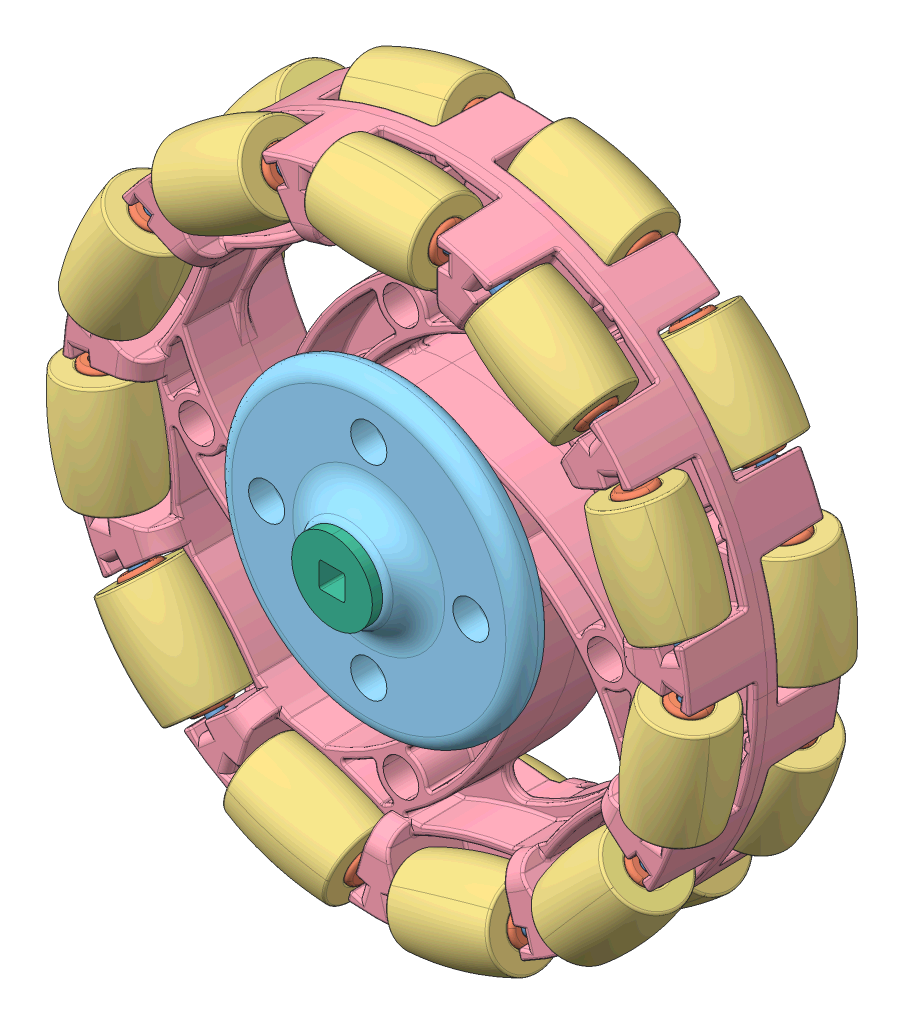
SolidWorks assembly Holo_Module_Omni_Wheel_Assembly, configuration Default. Lengths in mm.
Overall size (90.82 89.11 34).
95 component instances, 6 part files, 12 mates.
Components (placement in the parent):
- 3.25_ Omni-Directional Wheel (276-3526) part-1: 3.25_ Omni-Directional Wheel (276-3526) part [Default] at (20.7471 51.0724 74.1563) size (90.82 89.11 34)
  - 3.25_ Omni-Directional Wheel (276-3526) .step-1: 3.25_ Omni-Directional Wheel (276-3526) .step [Default] at origin size (90.82 89.11 34)
    - Roller Assembly.step-1: Roller Assembly.step [Default] at (-0.0014 35.9575 7.1) x (0 0.963098 -0.269151) z (-1 0 0) size (14.05 14.05 18.75)
      - 276-3526-001 Rev 1.step-1: 276-3526-001 Rev 1.step [Default] at origin size (2 2 18.75)
      - 276-3526-003 Rev 1.step-1: 276-3526-003 Rev 1.step [Default] at origin size (6.15 6.15 14.2)
      - 276-3526-002 Rev 1.step-1: 276-3526-002 Rev 1.step [Default] x (0 0 1) z (-0.908956 0.416893 0) size (13.2 10.6 10.6)
    - Roller Assembly.step-2: Roller Assembly.step [Default] at (-19.4287 30.2567 7.1) x (0.421057 -0.655178 0.627258) z (-0.841254 -0.540641 0) size (14.05 14.05 18.75)
      - 276-3526-001 Rev 1.step-1: 276-3526-001 Rev 1.step [Default] at origin size (2 2 18.75)
      - 276-3526-003 Rev 1.step-1: 276-3526-003 Rev 1.step [Default] at origin size (6.15 6.15 14.2)
      - 276-3526-002 Rev 1.step-1: 276-3526-002 Rev 1.step [Default] x (0 0 1) z (-0.908956 0.416893 0) size (13.2 10.6 10.6)
    - Roller Assembly.step-3: Roller Assembly.step [Default] at (-35.5935 -5.1038 7.1) x (0.979746 0.140866 -0.142315) z (0.142315 -0.989821 0) size (14.05 14.05 18.75)
      - 276-3526-001 Rev 1.step-1: 276-3526-001 Rev 1.step [Default] at origin size (2 2 18.75)
      - 276-3526-003 Rev 1.step-1: 276-3526-003 Rev 1.step [Default] at origin size (6.15 6.15 14.2)
      - 276-3526-002 Rev 1.step-1: 276-3526-002 Rev 1.step [Default] x (0 0 1) z (-0.908956 0.416893 0) size (13.2 10.6 10.6)
    - Roller Assembly.step-4: Roller Assembly.step [Default] at (-10.1434 -34.4972 7.1) x (0.079373 0.27032 -0.959493) z (0.959493 -0.281733 0) size (14.05 14.05 18.75)
      - 276-3526-001 Rev 1.step-1: 276-3526-001 Rev 1.step [Default] at origin size (2 2 18.75)
      - 276-3526-003 Rev 1.step-1: 276-3526-003 Rev 1.step [Default] at origin size (6.15 6.15 14.2)
      - 276-3526-002 Rev 1.step-1: 276-3526-002 Rev 1.step [Default] x (0 0 1) z (-0.908956 0.416893 0) size (13.2 10.6 10.6)
    - Roller Assembly.step-5: Roller Assembly.step [Default] at (27.166 -23.5574 7.1) x (-0.355209 0.30779 -0.882662) z (0.654861 0.75575 0) size (14.05 14.05 18.75)
      - 276-3526-001 Rev 1.step-1: 276-3526-001 Rev 1.step [Default] at origin size (2 2 18.75)
      - 276-3526-003 Rev 1.step-1: 276-3526-003 Rev 1.step [Default] at origin size (6.15 6.15 14.2)
      - 276-3526-002 Rev 1.step-1: 276-3526-002 Rev 1.step [Default] x (0 0 1) z (-0.908956 0.416893 0) size (13.2 10.6 10.6)
    - Roller Assembly.step-6: Roller Assembly.step [Default] at (32.7138 14.9249 7.1) x (0.89908 0.410596 0.151875) z (-0.415415 0.909632 0) size (14.05 14.05 18.75)
      - 276-3526-001 Rev 1.step-1: 276-3526-001 Rev 1.step [Default] at origin size (2 2 18.75)
      - 276-3526-003 Rev 1.step-1: 276-3526-003 Rev 1.step [Default] at origin size (6.15 6.15 14.2)
      - 276-3526-002 Rev 1.step-1: 276-3526-002 Rev 1.step [Default] x (0 0 1) z (-0.908956 0.416893 0) size (13.2 10.6 10.6)
    - Roller Assembly.step-7: Roller Assembly.step [Default] at (19.4515 30.242 7.1) x (0.194707 0.302971 0.932898) z (-0.841254 0.540641 0) size (14.05 14.05 18.75)
      - 276-3526-001 Rev 1.step-1: 276-3526-001 Rev 1.step [Default] at origin size (2 2 18.75)
      - 276-3526-003 Rev 1.step-1: 276-3526-003 Rev 1.step [Default] at origin size (6.15 6.15 14.2)
      - 276-3526-002 Rev 1.step-1: 276-3526-002 Rev 1.step [Default] x (0 0 1) z (-0.908956 0.416893 0) size (13.2 10.6 10.6)
    - Roller Assembly.step-8: Roller Assembly.step [Default] at (-32.7025 14.9497 7.1) x (0.82743 -0.377875 0.415415) z (-0.415415 -0.909632 0) size (14.05 14.05 18.75)
      - 276-3526-001 Rev 1.step-1: 276-3526-001 Rev 1.step [Default] at origin size (2 2 18.75)
      - 276-3526-003 Rev 1.step-1: 276-3526-003 Rev 1.step [Default] at origin size (6.15 6.15 14.2)
      - 276-3526-002 Rev 1.step-1: 276-3526-002 Rev 1.step [Default] x (0 0 1) z (-0.908956 0.416893 0) size (13.2 10.6 10.6)
    - Roller Assembly.step-9: Roller Assembly.step [Default] at (-27.1838 -23.5369 7.1) x (0.578931 0.501646 -0.642799) z (0.654861 -0.75575 0) size (14.05 14.05 18.75)
      - 276-3526-001 Rev 1.step-1: 276-3526-001 Rev 1.step [Default] at origin size (2 2 18.75)
      - 276-3526-003 Rev 1.step-1: 276-3526-003 Rev 1.step [Default] at origin size (6.15 6.15 14.2)
      - 276-3526-002 Rev 1.step-1: 276-3526-002 Rev 1.step [Default] x (0 0 1) z (-0.908956 0.416893 0) size (13.2 10.6 10.6)
    - Roller Assembly.step-10: Roller Assembly.step [Default] at (10.1174 -34.5048 7.1) x (0.079373 -0.27032 -0.959493) z (0.959493 0.281733 0) size (14.05 14.05 18.75)
      - 276-3526-001 Rev 1.step-1: 276-3526-001 Rev 1.step [Default] at origin size (2 2 18.75)
      - 276-3526-003 Rev 1.step-1: 276-3526-003 Rev 1.step [Default] at origin size (6.15 6.15 14.2)
      - 276-3526-002 Rev 1.step-1: 276-3526-002 Rev 1.step [Default] x (0 0 1) z (-0.908956 0.416893 0) size (13.2 10.6 10.6)
    - Roller Assembly.step-11: Roller Assembly.step [Default] at (35.5896 -5.1307 7.1) x (0.988515 -0.142127 -0.05136) z (0.142315 0.989821 0) size (14.05 14.05 18.75)
      - 276-3526-001 Rev 1.step-1: 276-3526-001 Rev 1.step [Default] at origin size (2 2 18.75)
      - 276-3526-003 Rev 1.step-1: 276-3526-003 Rev 1.step [Default] at origin size (6.15 6.15 14.2)
      - 276-3526-002 Rev 1.step-1: 276-3526-002 Rev 1.step [Default] x (0 0 1) z (-0.908956 0.416893 0) size (13.2 10.6 10.6)
    - Roller Assembly.step-12: Roller Assembly.step [Default] at (10.1434 34.4972 -7.1) x (0.083119 0.283078 -0.955489) z (0.959493 -0.281733 0) size (14.05 14.05 18.75)
      - 276-3526-001 Rev 1.step-1: 276-3526-001 Rev 1.step [Default] at origin size (2 2 18.75)
      - 276-3526-003 Rev 1.step-1: 276-3526-003 Rev 1.step [Default] at origin size (6.15 6.15 14.2)
      - 276-3526-002 Rev 1.step-1: 276-3526-002 Rev 1.step [Default] x (0 0 1) z (-0.908956 0.416893 0) size (13.2 10.6 10.6)
    - Roller Assembly.step-13: Roller Assembly.step [Default] at (27.1838 23.5369 -7.1) x (0.582526 0.504762 -0.637086) z (0.654861 -0.75575 0) size (14.05 14.05 18.75)
      - 276-3526-001 Rev 1.step-1: 276-3526-001 Rev 1.step [Default] at origin size (2 2 18.75)
      - 276-3526-003 Rev 1.step-1: 276-3526-003 Rev 1.step [Default] at origin size (6.15 6.15 14.2)
      - 276-3526-002 Rev 1.step-1: 276-3526-002 Rev 1.step [Default] x (0 0 1) z (-0.908956 0.416893 0) size (13.2 10.6 10.6)
    - Roller Assembly.step-14: Roller Assembly.step [Default] at (35.5935 5.1038 -7.1) x (0.926341 0.133188 -0.352355) z (0.142315 -0.989821 0) size (14.05 14.05 18.75)
      - 276-3526-001 Rev 1.step-1: 276-3526-001 Rev 1.step [Default] at origin size (2 2 18.75)
      - 276-3526-003 Rev 1.step-1: 276-3526-003 Rev 1.step [Default] at origin size (6.15 6.15 14.2)
      - 276-3526-002 Rev 1.step-1: 276-3526-002 Rev 1.step [Default] x (0 0 1) z (-0.908956 0.416893 0) size (13.2 10.6 10.6)
    - Roller Assembly.step-15: Roller Assembly.step [Default] at (32.7025 -14.9497 -7.1) x (0.897398 -0.409828 0.163453) z (-0.415415 -0.909632 0) size (14.05 14.05 18.75)
      - 276-3526-001 Rev 1.step-1: 276-3526-001 Rev 1.step [Default] at origin size (2 2 18.75)
      - 276-3526-003 Rev 1.step-1: 276-3526-003 Rev 1.step [Default] at origin size (6.15 6.15 14.2)
      - 276-3526-002 Rev 1.step-1: 276-3526-002 Rev 1.step [Default] x (0 0 1) z (-0.908956 0.416893 0) size (13.2 10.6 10.6)
    - Roller Assembly.step-16: Roller Assembly.step [Default] at (19.4287 -30.2567 -7.1) x (0.277612 -0.431972 0.858098) z (-0.841254 -0.540641 0) size (14.05 14.05 18.75)
      - 276-3526-001 Rev 1.step-1: 276-3526-001 Rev 1.step [Default] at origin size (2 2 18.75)
      - 276-3526-003 Rev 1.step-1: 276-3526-003 Rev 1.step [Default] at origin size (6.15 6.15 14.2)
      - 276-3526-002 Rev 1.step-1: 276-3526-002 Rev 1.step [Default] x (0 0 1) z (-0.908956 0.416893 0) size (13.2 10.6 10.6)
    - Roller Assembly.step-17: Roller Assembly.step [Default] at (-0.0136 -35.9575 -7.1) x (0 -0.239919 0.970793) z (-1 0 0) size (14.05 14.05 18.75)
      - 276-3526-001 Rev 1.step-1: 276-3526-001 Rev 1.step [Default] at origin size (2 2 18.75)
      - 276-3526-003 Rev 1.step-1: 276-3526-003 Rev 1.step [Default] at origin size (6.15 6.15 14.2)
      - 276-3526-002 Rev 1.step-1: 276-3526-002 Rev 1.step [Default] x (0 0 1) z (-0.908956 0.416893 0) size (13.2 10.6 10.6)
    - Roller Assembly.step-18: Roller Assembly.step [Default] at (-19.4515 -30.242 -7.1) x (0.31008 0.482494 0.819176) z (-0.841254 0.540641 0) size (14.05 14.05 18.75)
      - 276-3526-001 Rev 1.step-1: 276-3526-001 Rev 1.step [Default] at origin size (2 2 18.75)
      - 276-3526-003 Rev 1.step-1: 276-3526-003 Rev 1.step [Default] at origin size (6.15 6.15 14.2)
      - 276-3526-002 Rev 1.step-1: 276-3526-002 Rev 1.step [Default] x (0 0 1) z (-0.908956 0.416893 0) size (13.2 10.6 10.6)
    - Roller Assembly.step-19: Roller Assembly.step [Default] at (-32.7138 -14.9249 -7.1) x (0.58758 0.268339 0.763377) z (-0.415415 0.909632 0) size (14.05 14.05 18.75)
      - 276-3526-001 Rev 1.step-1: 276-3526-001 Rev 1.step [Default] at origin size (2 2 18.75)
      - 276-3526-003 Rev 1.step-1: 276-3526-003 Rev 1.step [Default] at origin size (6.15 6.15 14.2)
      - 276-3526-002 Rev 1.step-1: 276-3526-002 Rev 1.step [Default] x (0 0 1) z (-0.908956 0.416893 0) size (13.2 10.6 10.6)
    - Roller Assembly.step-20: Roller Assembly.step [Default] at (-35.5896 5.1307 -7.1) x (0.965498 -0.138818 0.220323) z (0.142315 0.989821 0) size (14.05 14.05 18.75)
      - 276-3526-001 Rev 1.step-1: 276-3526-001 Rev 1.step [Default] at origin size (2 2 18.75)
      - 276-3526-003 Rev 1.step-1: 276-3526-003 Rev 1.step [Default] at origin size (6.15 6.15 14.2)
      - 276-3526-002 Rev 1.step-1: 276-3526-002 Rev 1.step [Default] x (0 0 1) z (-0.908956 0.416893 0) size (13.2 10.6 10.6)
    - Roller Assembly.step-21: Roller Assembly.step [Default] at (-27.166 23.5574 -7.1) x (0.75327 -0.652712 -0.080935) z (0.654861 0.75575 0) size (14.05 14.05 18.75)
      - 276-3526-001 Rev 1.step-1: 276-3526-001 Rev 1.step [Default] at origin size (2 2 18.75)
      - 276-3526-003 Rev 1.step-1: 276-3526-003 Rev 1.step [Default] at origin size (6.15 6.15 14.2)
      - 276-3526-002 Rev 1.step-1: 276-3526-002 Rev 1.step [Default] x (0 0 1) z (-0.908956 0.416893 0) size (13.2 10.6 10.6)
    - Roller Assembly.step-22: Roller Assembly.step [Default] at (-10.1174 34.5048 -7.1) x (0.123782 -0.421563 -0.898311) z (0.959493 0.281733 0) size (14.05 14.05 18.75)
      - 276-3526-001 Rev 1.step-1: 276-3526-001 Rev 1.step [Default] at origin size (2 2 18.75)
      - 276-3526-003 Rev 1.step-1: 276-3526-003 Rev 1.step [Default] at origin size (6.15 6.15 14.2)
      - 276-3526-002 Rev 1.step-1: 276-3526-002 Rev 1.step [Default] x (0 0 1) z (-0.908956 0.416893 0) size (13.2 10.6 10.6)
    - 276-3526-004 Rev 1.step-1: 276-3526-004 Rev 1.step [Default] at origin size (78.5 78.5 19.07)
- Wheel_Spacer-1: Wheel_Spacer [Default] at (20.7471 51.0724 80.5063) size (38.1 38.1 7.3)
- Wheel_Spacer-2: Wheel_Spacer [Default] at (20.7471 51.0724 67.8063) x (1 0 0) z (0 0 -1) size (38.1 38.1 7.3)
- Metal Shaft Inserts (276-3881-002)-1: Metal Shaft Inserts (276-3881-002) [Default] at (20.7471 51.0724 89.0763) x (1 0 0) z (0 1 0) size (10.03 5.08 10.03)
- Metal Shaft Inserts (276-3881-002)-2: Metal Shaft Inserts (276-3881-002) [Default] at (20.7471 51.0724 59.2363) x (1 0 0) z (0 -1 0) size (10.03 5.08 10.03)
Mates (geometry in assembly coordinates):
- Concentric1: concentric anti-aligned: cylinder of 3.25_ Omni-Directional Wheel (276-3526) part-1/3.25_ Omni-Directional Wheel (276-3526) .step-1/276-3526-004 Rev 1.step-1 through (20.7471 63.7724 64.6313) axis (0 0 1) radius 2.2225; cylinder of Wheel_Spacer-1 through (20.7471 63.7724 84.5063) axis (0 0 -1) radius 2.25
- Concentric2: concentric anti-aligned: cylinder of 3.25_ Omni-Directional Wheel (276-3526) part-1/3.25_ Omni-Directional Wheel (276-3526) .step-1/276-3526-004 Rev 1.step-1 through (20.7471 38.3724 64.6313) axis (0 0 1) radius 2.2225; cylinder of Wheel_Spacer-1 through (20.7471 38.3724 84.5063) axis (0 0 -1) radius 2.25
- Coincident1: coincident anti-aligned: plane of 3.25_ Omni-Directional Wheel (276-3526) part-1/3.25_ Omni-Directional Wheel (276-3526) .step-1/276-3526-004 Rev 1.step-1 through (20.7471 51.0724 80.5063) normal (0 0 1); plane of Wheel_Spacer-1 through (20.7471 51.0724 80.5063) normal (0 0 -1)
- Concentric3: concentric aligned: cylinder of 3.25_ Omni-Directional Wheel (276-3526) part-1/3.25_ Omni-Directional Wheel (276-3526) .step-1/276-3526-004 Rev 1.step-1 through (8.0471 51.0724 64.6313) axis (0 0 1) radius 2.2225; cylinder of Wheel_Spacer-2 through (8.0471 51.0724 63.8063) axis (0 0 1) radius 2.25
- Concentric4: concentric aligned: cylinder of 3.25_ Omni-Directional Wheel (276-3526) part-1/3.25_ Omni-Directional Wheel (276-3526) .step-1/276-3526-004 Rev 1.step-1 through (33.4471 51.0724 64.6313) axis (0 0 1) radius 2.2225; cylinder of Wheel_Spacer-2 through (33.4471 51.0724 63.8063) axis (0 0 1) radius 2.25
- Coincident2: coincident anti-aligned: plane of 3.25_ Omni-Directional Wheel (276-3526) part-1/3.25_ Omni-Directional Wheel (276-3526) .step-1/276-3526-004 Rev 1.step-1 through (20.7471 51.0724 67.8063) normal (0 0 -1); plane of Wheel_Spacer-2 through (20.7471 51.0724 67.8063) normal (0 0 1)
- Coincident3: coincident anti-aligned: plane of Wheel_Spacer-1 through (20.7471 51.0724 87.8063) normal (0 0 1); plane of Metal Shaft Inserts (276-3881-002)-1 through (20.7471 51.0724 87.8063) normal (0 0 -1)
- Concentric5: concentric anti-aligned: circle of Wheel_Spacer-1; circle of Metal Shaft Inserts (276-3881-002)-1
- Coincident4: coincident anti-aligned: plane of Wheel_Spacer-2 through (20.7471 51.0724 60.5063) normal (0 0 -1); plane of Metal Shaft Inserts (276-3881-002)-2 through (20.7471 51.0724 60.5063) normal (0 0 1)
- Concentric6: concentric anti-aligned: circle of Wheel_Spacer-2; circle of Metal Shaft Inserts (276-3881-002)-2
- Parallel1: parallel aligned: plane of Wheel_Spacer-2 through (20.7471 47.8724 63.8063) normal (0 1 0); plane of Metal Shaft Inserts (276-3881-002)-2 through (19.1596 49.4849 64.3163) normal (0 1 0)
- Parallel2: parallel aligned: plane of Wheel_Spacer-1 through (20.7471 47.8724 84.5063) normal (0 1 0); plane of Metal Shaft Inserts (276-3881-002)-1 through (19.1596 49.4849 83.9963) normal (0 1 0)
